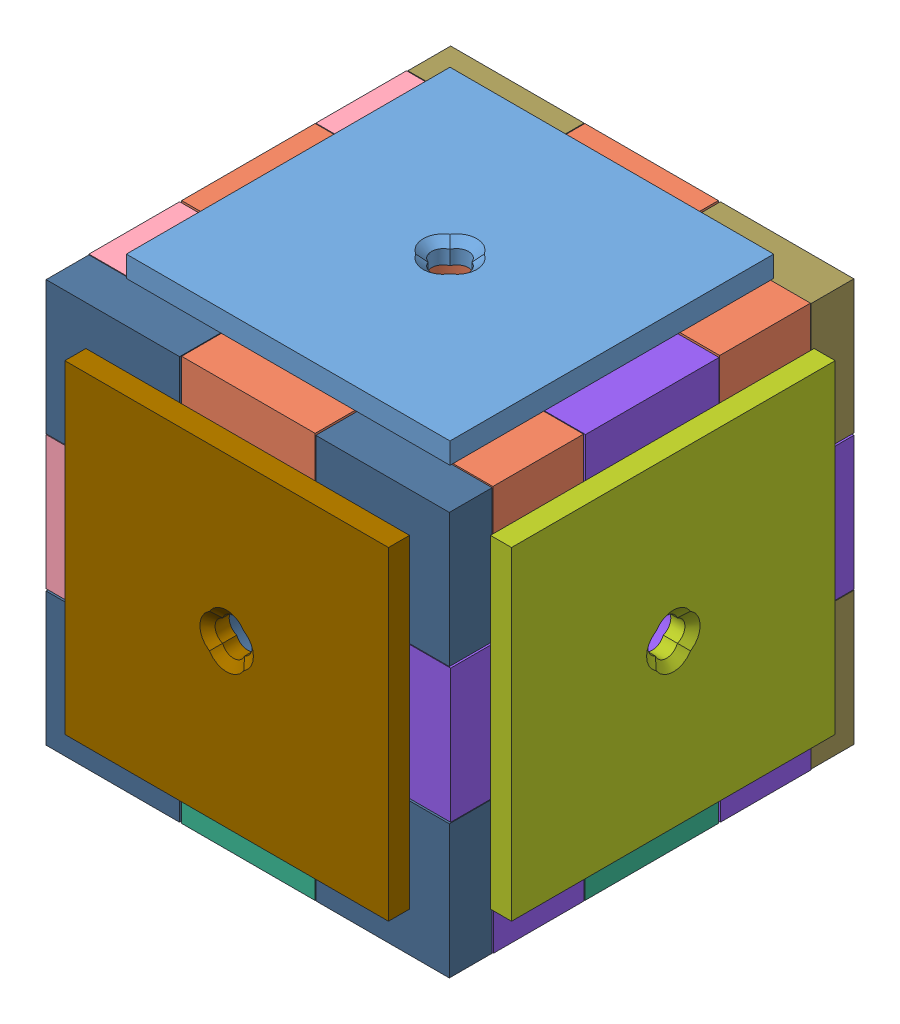
SolidWorks assembly cube_, configuration cube12. Lengths in mm.
Overall size (33.65 33.65 33.65).
12 component instances, 12 part files, 6 mates.
Components (placement in the parent):
- panel_R^cube_-13: panel_R^cube_ [cube01] x (-1 0 0) z (0 0 1) (virtual)
- acrylic_R^cube_-1: acrylic_R^cube_ [A] at origin (virtual)
- panel_O^cube_-8: panel_O^cube_ [cube01] x (0 -1 0) z (0 0 1) (virtual)
- acrylic_O^cube_-23: acrylic_O^cube_ [A] x (0 1 0) z (0 0 1) (virtual)
- panel_Y^cube_-9: panel_Y^cube_ [cube01] at origin (virtual)
- acrylic_Y^cube_-24: acrylic_Y^cube_ [A] x (-1 0 0) z (0 0 1) (virtual)
- panel_G^cube_-10: panel_G^cube_ [cube01] x (0 1 0) z (0 0 1) (virtual)
- acrylic_G^cube_-25: acrylic_G^cube_ [A] x (0 -1 0) z (0 0 1) (virtual)
- panel_C^cube_-11: panel_C^cube_ [cube01] x (-1 0 0) z (0 -1 0) (virtual)
- acrylic_C^cube_-26: acrylic_C^cube_ [B] x (1 0 0) z (0 -1 0) (virtual)
- panel_B^cube_-13: panel_B^cube_ [cube01] x (-1 0 0) z (0 1 0) (virtual)
- acrylic_B^cube_-27: acrylic_B^cube_ [B] x (1 0 0) z (0 1 0) (virtual)
Mates (geometry in assembly coordinates):
- Coincident1: coincident aligned: plane of panel_R^cube_-13 through (0 0 0) normal (0 0 1); plane of assembly through (0 0 0) normal (0 0 1)
- Coincident2: coincident anti-aligned: plane of panel_R^cube_-13; plane of assembly through (0 0 0) normal (1 0 0)
- Coincident3: coincident anti-aligned: plane of panel_R^cube_-13; plane of assembly through (0 0 0) normal (0 1 0)
- Coincident4: coincident aligned: plane of acrylic_R^cube_-1 through (0 0 0) normal (0 0 1); plane of assembly through (0 0 0) normal (0 0 1)
- Coincident5: coincident aligned: plane of acrylic_R^cube_-1 through (0 0 0) normal (1 0 0); plane of assembly through (0 0 0) normal (1 0 0)
- Coincident6: coincident aligned: plane of ? through (0 0 0) normal (0 1 0); plane of assembly through (0 0 0) normal (0 1 0)
